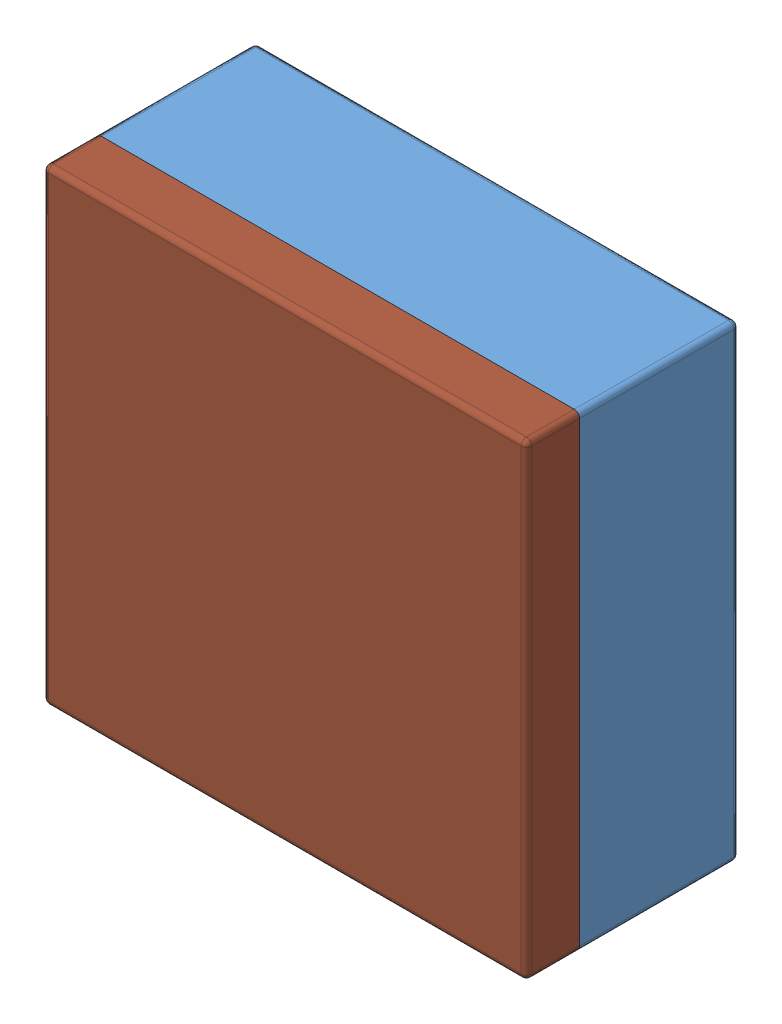
SolidWorks assembly Assem1, configuration Default. Lengths in mm.
Overall size (91 88 40).
617 component instances, 138 part files, 2 mates.
Components (placement in the parent):
- Assem147-1: Assem147 [Default] at (118.0608 24.9039 43.2392) size (91 88 30)
  - 2nd below-1: 2nd below [Default] at (-134.3508 -23.6695 15.6533) size (91 88 30)
  - Main Controller.step-1: Main Controller.step [Default] at (-5.5498 -47.3965 22.6108) x (0 1 0) z (0 0 1) size (83.62 86.87 19.5)
    - Board.step-1: Board.step [Default] at origin size (78.99 86.87 0.41)
      - Open CASCADE STEP translator 6.8 1.1.1.step-1: Open CASCADE STEP translator 6.8 1.1.1.step [Default] at (0 0 -0.4115) size (78.99 86.87 0.41)
    - IC2.step-1: IC2.step [Default] at origin size (3 4.93 1.1)
      - 6352354192.step-1: 6352354192.step [Default] at (37.973 87.63 0.69) x (1 0 0) z (0 -1 0) size (3 1.1 4.93)
        - BODY-SO.step-1: BODY-SO.step [Default] at origin size (3 1 3)
        - LEAD-SO.step-1: LEAD-SO.step [Default] at (1 -0.44 1.9) size (0.22 0.69 0.96)
        - LEAD-SO.step-2: LEAD-SO.step [Default] at (0.5 -0.44 1.9) size (0.22 0.69 0.96)
        - LEAD-SO.step-3: LEAD-SO.step [Default] at (0 -0.44 1.9) size (0.22 0.69 0.96)
        - LEAD-SO.step-4: LEAD-SO.step [Default] at (-0.5 -0.44 1.9) size (0.22 0.69 0.96)
        - LEAD-SO.step-5: LEAD-SO.step [Default] at (-1 -0.44 1.9) size (0.22 0.69 0.96)
        - LEAD-SO.step-6: LEAD-SO.step [Default] at (1 -0.44 -1.9) x (-1 0 0) z (0 0 -1) size (0.22 0.69 0.96)
        - LEAD-SO.step-7: LEAD-SO.step [Default] at (0.5 -0.44 -1.9) x (-1 0 0) z (0 0 -1) size (0.22 0.69 0.96)
        - LEAD-SO.step-8: LEAD-SO.step [Default] at (0 -0.44 -1.9) x (-1 0 0) z (0 0 -1) size (0.22 0.69 0.96)
        - LEAD-SO.step-9: LEAD-SO.step [Default] at (-0.5 -0.44 -1.9) x (-1 0 0) z (0 0 -1) size (0.22 0.69 0.96)
        - LEAD-SO.step-10: LEAD-SO.step [Default] at (-1 -0.44 -1.9) x (-1 0 0) z (0 0 -1) size (0.22 0.69 0.96)
    - S2.step-1: S2.step [Default] at origin size (4.38 3.7 1.8)
      - 6352354672.step-1: 6352354672.step [Default] at (30.053 53.017 0) size (4.38 3.7 1.8)
        - Body.step-1: Body.step [Default] at (0 0 0.1) size (3.82 3.4 1.7)
        - Pins.step-1: Pins.step [Default] at origin size (4.38 3.7 0.1)
    - S1.step-1: S1.step [Default] at origin size (4.38 3.7 1.8)
      - 6352354672.step-1: 6352354672.step [Default] at (30.053 62.1012 0) size (4.38 3.7 1.8)
        - Body.step-1: Body.step [Default] at (0 0 0.1) size (3.82 3.4 1.7)
        - Pins.step-1: Pins.step [Default] at origin size (4.38 3.7 0.1)
    - DS2.step-1: DS2.step [Default] at origin size (1.6 0.8 0.9)
      - 6357174448.step-1: 6357174448.step [Default] at (51.31 84.836 0.4) size (1.1 0.8 0.5)
        - Extruded.step-1: Extruded.step [Default] at origin size (1.1 0.8 0.5)
      - 6357174288.step-1: 6357174288.step [Default] at (51.31 84.836 0) size (1.6 0.8 0.4)
        - Extruded-0.step-1: Extruded-0.step [Default] at origin size (1.6 0.8 0.4)
    - DS1.step-1: DS1.step [Default] at origin size (0.8 1.6 0.9)
      - 6357175488.step-1: 6357175488.step [Default] at (71.8819 81.917 0.4) size (0.8 1.1 0.5)
        - Extruded-1.step-1: Extruded-1.step [Default] at origin size (0.8 1.1 0.5)
      - 6357175328.step-1: 6357175328.step [Default] at (71.8819 81.917 0) size (0.8 1.6 0.4)
        - Extruded-2.step-1: Extruded-2.step [Default] at origin size (0.8 1.6 0.4)
    - P1.step-1: P1.step [Default] at origin size (7.9 4.5 9.4)
      - 6357176688.step-1: 6357176688.step [Default] at (78.67 45.298 0) size (3.15 1.45 6)
        - Extruded-3.step-1: Extruded-3.step [Default] at origin size (3.15 1.45 6)
      - 6357176528.step-1: 6357176528.step [Default] at (79.92 44.173 0) size (0.65 0.8 4.1)
        - Extruded-4.step-1: Extruded-4.step [Default] at origin size (0.65 0.8 4.1)
      - 6357176528.step-2: 6357176528.step [Default] at (72.67 44.173 0) size (0.65 0.8 4.1)
        - Extruded-4.step-1: Extruded-4.step [Default] at origin size (0.65 0.8 4.1)
      - 6357176288.step-1: 6357176288.step [Default] at (73.92 45.298 0) size (3.15 1.45 6)
        - Extruded-5.step-1: Extruded-5.step [Default] at origin size (3.15 1.45 6)
      - 6357176128.step-1: 6357176128.step [Default] at (76.295 42.648 0) size (7.9 2.25 6)
        - Extruded-6.step-1: Extruded-6.step [Default] at origin size (7.9 2.25 6)
      - 6357175968.step-1: 6357175968.step [Default] at (76.295 43.973 0) size (6.6 4.1 1.75)
        - Extruded-7.step-1: Extruded-7.step [Default] at origin size (6.6 4.1 1.75)
      - 6357175808.step-1: 6357175808.step [Default] at (76.295 44.323 -3.4) size (0.5 0.5 8.45)
        - Extruded-8.step-1: Extruded-8.step [Default] at origin size (0.5 0.5 8.45)
      - 6357175808.step-2: 6357175808.step [Default] at (74.295 44.323 -3.4) size (0.5 0.5 8.45)
        - Extruded-8.step-1: Extruded-8.step [Default] at origin size (0.5 0.5 8.45)
      - 6357175808.step-3: 6357175808.step [Default] at (78.295 44.323 -3.4) size (0.5 0.5 8.45)
        - Extruded-8.step-1: Extruded-8.step [Default] at origin size (0.5 0.5 8.45)
    - P2.step-1: P2.step [Default] at origin size (7.9 4.5 9.4)
      - 6357176688.step-1: 6357176688.step [Default] at (64.478 45.213 0) size (3.15 1.45 6)
        - Extruded-3.step-1: Extruded-3.step [Default] at origin size (3.15 1.45 6)
      - 6357176528.step-1: 6357176528.step [Default] at (65.728 44.088 0) size (0.65 0.8 4.1)
        - Extruded-4.step-1: Extruded-4.step [Default] at origin size (0.65 0.8 4.1)
      - 6357176528.step-2: 6357176528.step [Default] at (58.478 44.088 0) size (0.65 0.8 4.1)
        - Extruded-4.step-1: Extruded-4.step [Default] at origin size (0.65 0.8 4.1)
      - 6357176288.step-1: 6357176288.step [Default] at (59.728 45.213 0) size (3.15 1.45 6)
        - Extruded-5.step-1: Extruded-5.step [Default] at origin size (3.15 1.45 6)
      - 6357176128.step-1: 6357176128.step [Default] at (62.103 42.563 0) size (7.9 2.25 6)
        - Extruded-6.step-1: Extruded-6.step [Default] at origin size (7.9 2.25 6)
      - 6357175968.step-1: 6357175968.step [Default] at (62.103 43.888 0) size (6.6 4.1 1.75)
        - Extruded-7.step-1: Extruded-7.step [Default] at origin size (6.6 4.1 1.75)
      - 6357175808.step-1: 6357175808.step [Default] at (62.103 44.238 -3.4) size (0.5 0.5 8.45)
        - Extruded-8.step-1: Extruded-8.step [Default] at origin size (0.5 0.5 8.45)
      - 6357175808.step-2: 6357175808.step [Default] at (60.103 44.238 -3.4) size (0.5 0.5 8.45)
        - Extruded-8.step-1: Extruded-8.step [Default] at origin size (0.5 0.5 8.45)
      - 6357175808.step-3: 6357175808.step [Default] at (64.103 44.238 -3.4) size (0.5 0.5 8.45)
        - Extruded-8.step-1: Extruded-8.step [Default] at origin size (0.5 0.5 8.45)
    - K1.step-1: K1.step [Default] at origin size (15 19 19.5)
      - 6352352272.step-1: 6352352272.step [Default] at (79.2542 59.744 15.04) x (0 1 0) z (0 0 -1) size (19 15 19.5)
    - K2.step-1: K2.step [Default] at origin size (15 19 19.5)
      - 6352352272.step-1: 6352352272.step [Default] at (63.246 59.744 15.04) x (0 1 0) z (0 0 -1) size (19 15 19.5)
    - U5.step-1: U5.step [Default] at origin size (6.42 7.8 1)
      - PW0024AakaMTC24.step-1: PW0024AakaMTC24.step [Default] at (53.9751 104.7751 0.624) x (0 1 0) z (1 0 0) size (7.8 1 6.42)
        - BODY_MTC24.step-1: BODY_MTC24.step [Default] at origin size (7.8 0.9 4.4)
        - LEAD_MTC24.step-1: LEAD_MTC24.step [Default] at (3.575 -0.3725 -2.6) x (-1 0 0) z (0 0 -1) size (0.24 0.62 1.01)
        - LEAD_MTC24.step-2: LEAD_MTC24.step [Default] at (2.925 -0.3725 -2.6) x (-1 0 0) z (0 0 -1) size (0.24 0.62 1.01)
        - LEAD_MTC24.step-3: LEAD_MTC24.step [Default] at (2.275 -0.3725 -2.6) x (-1 0 0) z (0 0 -1) size (0.24 0.62 1.01)
        - LEAD_MTC24.step-4: LEAD_MTC24.step [Default] at (1.625 -0.3725 -2.6) x (-1 0 0) z (0 0 -1) size (0.24 0.62 1.01)
        - LEAD_MTC24.step-5: LEAD_MTC24.step [Default] at (0.975 -0.3725 -2.6) x (-1 0 0) z (0 0 -1) size (0.24 0.62 1.01)
        - LEAD_MTC24.step-6: LEAD_MTC24.step [Default] at (0.325 -0.3725 -2.6) x (-1 0 0) z (0 0 -1) size (0.24 0.62 1.01)
        - LEAD_MTC24.step-7: LEAD_MTC24.step [Default] at (-0.325 -0.3725 -2.6) x (-1 0 0) z (0 0 -1) size (0.24 0.62 1.01)
        - LEAD_MTC24.step-8: LEAD_MTC24.step [Default] at (-0.975 -0.3725 -2.6) x (-1 0 0) z (0 0 -1) size (0.24 0.62 1.01)
        - LEAD_MTC24.step-9: LEAD_MTC24.step [Default] at (-1.625 -0.3725 -2.6) x (-1 0 0) z (0 0 -1) size (0.24 0.62 1.01)
        - LEAD_MTC24.step-10: LEAD_MTC24.step [Default] at (-2.275 -0.3725 -2.6) x (-1 0 0) z (0 0 -1) size (0.24 0.62 1.01)
        - LEAD_MTC24.step-11: LEAD_MTC24.step [Default] at (-2.925 -0.3725 -2.6) x (-1 0 0) z (0 0 -1) size (0.24 0.62 1.01)
        - LEAD_MTC24.step-12: LEAD_MTC24.step [Default] at (-3.575 -0.3725 -2.6) x (-1 0 0) z (0 0 -1) size (0.24 0.62 1.01)
        - LEAD_MTC24.step-13: LEAD_MTC24.step [Default] at (3.575 -0.3725 2.6) size (0.24 0.62 1.01)
        - LEAD_MTC24.step-14: LEAD_MTC24.step [Default] at (2.925 -0.3725 2.6) size (0.24 0.62 1.01)
        - LEAD_MTC24.step-15: LEAD_MTC24.step [Default] at (2.275 -0.3725 2.6) size (0.24 0.62 1.01)
        - LEAD_MTC24.step-16: LEAD_MTC24.step [Default] at (1.625 -0.3725 2.6) size (0.24 0.62 1.01)
        - LEAD_MTC24.step-17: LEAD_MTC24.step [Default] at (0.975 -0.3725 2.6) size (0.24 0.62 1.01)
        - LEAD_MTC24.step-18: LEAD_MTC24.step [Default] at (0.325 -0.3725 2.6) size (0.24 0.62 1.01)
        - LEAD_MTC24.step-19: LEAD_MTC24.step [Default] at (-0.325 -0.3725 2.6) size (0.24 0.62 1.01)
        - LEAD_MTC24.step-20: LEAD_MTC24.step [Default] at (-0.975 -0.3725 2.6) size (0.24 0.62 1.01)
        - LEAD_MTC24.step-21: LEAD_MTC24.step [Default] at (-1.625 -0.3725 2.6) size (0.24 0.62 1.01)
        - LEAD_MTC24.step-22: LEAD_MTC24.step [Default] at (-2.275 -0.3725 2.6) size (0.24 0.62 1.01)
        - LEAD_MTC24.step-23: LEAD_MTC24.step [Default] at (-2.925 -0.3725 2.6) size (0.24 0.62 1.01)
        - LEAD_MTC24.step-24: LEAD_MTC24.step [Default] at (-3.575 -0.3725 2.6) size (0.24 0.62 1.01)
    - U4.step-1: U4.step [Default] at origin size (4.9 6 1.76)
      - IC_Texas_Instruments_ISO7220ADR_eec.step-1: IC_Texas_Instruments_ISO7220ADR_eec.step [Default] at (51.943 77.597 0) x (0 1 0) z (0 0 1) size (6 4.9 1.76)
        - IC_BODY.step-1: IC_BODY.step [Default] at (0 0 0.25) x (0 -1 0) z (0 0 1) size (4.9 3.9 1.5)
        - circle.step-1: circle.step [Default] at (-1.0726 1.9393 1.751) x (1 0 0) z (0 0 -1) size (0.4 0.4 0)
        - IC_LEG.step-1: IC_LEG.step [Default] at (-3 2.1095 0) x (1 0 0) z (0 -1 0) size (1.15 1.11 0.41)
        - IC_LEG.step-2: IC_LEG.step [Default] at (-3 0.8395 0) x (1 0 0) z (0 -1 0) size (1.15 1.11 0.41)
        - IC_LEG.step-3: IC_LEG.step [Default] at (-3 -0.4305 0) x (1 0 0) z (0 -1 0) size (1.15 1.11 0.41)
        - IC_LEG.step-4: IC_LEG.step [Default] at (-3 -1.7005 0) x (1 0 0) z (0 -1 0) size (1.15 1.11 0.41)
        - Texas_Instruments.step-1: Texas_Instruments.step [Default] at (0.0232 -1.7093 1.75) size (3.04 0.71 0.02)
        - IC_LEG_MIR8.step-1: IC_LEG_MIR8.step [Default] at (3 2.1095 0) x (-1 0 0) z (0 1 0) size (1.15 1.11 0.41)
        - IC_LEG_MIR8.step-2: IC_LEG_MIR8.step [Default] at (3 0.8395 0) x (-1 0 0) z (0 1 0) size (1.15 1.11 0.41)
        - IC_LEG_MIR8.step-3: IC_LEG_MIR8.step [Default] at (3 -0.4305 0) x (-1 0 0) z (0 1 0) size (1.15 1.11 0.41)
        - IC_LEG_MIR8.step-4: IC_LEG_MIR8.step [Default] at (3 -1.7005 0) x (-1 0 0) z (0 1 0) size (1.15 1.11 0.41)
    - U3.step-1: U3.step [Default] at origin size (7.05 6.5 1.8)
      - IC_Advanced_Monolithic_Systems_AMS1117-3_3_eec.step-1: IC_Advanced_Monolithic_Systems_AMS1117-3_3_eec.step [Default] at (38.227 106.68 0) size (7.05 6.51 1.8)
        - 2.step-1: 2.step [Default] x (1 0 0) z (0 -1 0) size (7.05 1.2 5.34)
          - Open CASCADE STEP translator 6.8 1.13.1.2.1.step-1: Open CASCADE STEP translator 6.8 1.13.1.2.1.step [Default] at origin size (7.05 1.2 5.34)
          - Open CASCADE STEP translator 6.8 1.13.1.2.2.step-1: Open CASCADE STEP translator 6.8 1.13.1.2.2.step [Default] at origin
        - 1.step-1: 1.step [Default] at (0 0 0.74) x (0 1 0) z (0 0 1) size (6.51 3.5 1.06)
        - Notch_2.step-1: Notch_2.step [Default] at (-0.7251 1.7063 1.701) size (2.3 5.16 0.1)
    - U2.step-1: U2.step [Default] at origin size (4.9 6 1.63)
      - SOIC-8akaD0008AakaM08A.step-1: SOIC-8akaD0008AakaM08A.step [Default] at (69.5961 112.9199 1) x (1 0 0) z (0 -1 0) size (4.9 1.63 6)
        - M08A_ASM_82_ASM.step-1: M08A_ASM_82_ASM.step [Default] at origin size (4.9 1.63 6)
          - TIEBAR_M08A_2_ASM.step-1: TIEBAR_M08A_2_ASM.step [Default] at origin size (4.9 0.2 0.66)
            - MANIFOLD_SOLID_BREP_2784.step-1: MANIFOLD_SOLID_BREP_2784.step [Default] at origin size (0.2 0.2 0.15)
            - MANIFOLD_SOLID_BREP_2935.step-1: MANIFOLD_SOLID_BREP_2935.step [Default] at origin size (0.2 0.2 0.15)
            - MANIFOLD_SOLID_BREP_3086.step-1: MANIFOLD_SOLID_BREP_3086.step [Default] at origin size (0.2 0.2 0.15)
            - MANIFOLD_SOLID_BREP_3237.step-1: MANIFOLD_SOLID_BREP_3237.step [Default] at origin size (0.2 0.2 0.15)
          - BODY_M08A_35.step-1: BODY_M08A_35.step [Default] at origin size (4.9 1.45 3.9)
          - LEAD_M08A_57.step-1: LEAD_M08A_57.step [Default] at (1.905 -0.75 2.1732) size (0.38 1 1.05)
          - LEAD_M08A_57.step-2: LEAD_M08A_57.step [Default] at (0.635 -0.75 2.1732) size (0.38 1 1.05)
          - LEAD_M08A_57.step-3: LEAD_M08A_57.step [Default] at (-0.635 -0.75 2.1732) size (0.38 1 1.05)
          - LEAD_M08A_57.step-4: LEAD_M08A_57.step [Default] at (-1.905 -0.75 2.1732) size (0.38 1 1.05)
          - LEAD_M08A_57.step-5: LEAD_M08A_57.step [Default] at (1.905 -0.75 -2.1732) x (-1 0 0) z (0 0 -1) size (0.38 1 1.05)
          - LEAD_M08A_57.step-6: LEAD_M08A_57.step [Default] at (0.635 -0.75 -2.1732) x (-1 0 0) z (0 0 -1) size (0.38 1 1.05)
          - LEAD_M08A_57.step-7: LEAD_M08A_57.step [Default] at (-0.635 -0.75 -2.1732) x (-1 0 0) z (0 0 -1) size (0.38 1 1.05)
          - LEAD_M08A_57.step-8: LEAD_M08A_57.step [Default] at (-1.905 -0.75 -2.1732) x (-1 0 0) z (0 0 -1) size (0.38 1 1.05)
    - U1.step-1: U1.step [Default] at origin size (2.01 3.1 0.92)
      - IC_Texas_Instruments_TXS0102DCUR_eec.step-1: IC_Texas_Instruments_TXS0102DCUR_eec.step [Default] at (54.737 114.495 0) x (0 1 0) z (0 0 1) size (0.25 1.32 0.01)
      - IC_Texas_Instruments_TXS0102DCUR_eec-9.step-1: IC_Texas_Instruments_TXS0102DCUR_eec-9.step [Default] at (54.737 114.495 0) x (0 1 0) z (0 0 1) size (0.19 0.66 0.01)
      - IC_Texas_Instruments_TXS0102DCUR_eec-10.step-1: IC_Texas_Instruments_TXS0102DCUR_eec-10.step [Default] at (54.737 114.495 0) x (0 1 0) z (0 0 1) size (0.19 1.33 0.01)
      - IC_Texas_Instruments_TXS0102DCUR_eec-11.step-1: IC_Texas_Instruments_TXS0102DCUR_eec-11.step [Default] at (54.737 114.495 0) x (0 1 0) z (0 0 1) size (0.3 0.3 0.01)
      - IC_Texas_Instruments_TXS0102DCUR_eec-12.step-1: IC_Texas_Instruments_TXS0102DCUR_eec-12.step [Default] at (54.737 114.495 0) x (0 1 0) z (0 0 1) size (3.1 1.71 0.56)
      - IC_Texas_Instruments_TXS0102DCUR_eec-13.step-1: IC_Texas_Instruments_TXS0102DCUR_eec-13.step [Default] at (54.737 114.495 0) x (0 1 0) z (0 0 1) size (2.31 2.01 0.8)
    - R23.step-1: R23.step [Default] at origin size (0.8 1.6 0.56)
      - Res_Panasonic_Electronic_Components_ERA-3ARB202V_eec.step-1: Res_Panasonic_Electronic_Components_ERA-3ARB202V_eec.step [Default] at (70.739 75.309 0) x (0 -1 0) z (0 0 1) size (1.6 0.8 0.56)
        - 1-14.step-1: 1-14.step [Default] at origin size (1.52 0.8 0.47)
        - 2-15.step-1: 2-15.step [Default] at origin size (1.08 0.8 0.04)
        - 3.step-1: 3.step [Default] at origin size (1.6 0.8 0.55)
        - Panasonic_Logo.step-1: Panasonic_Logo.step [Default] at (-0.1032 0.2046 0.451) size (0.41 0.06 0.11)
    - R22.step-1: R22.step [Default] at origin size (0.8 1.6 0.56)
      - Res_Panasonic_Electronic_Components_ERA-3ARB202V_eec.step-1: Res_Panasonic_Electronic_Components_ERA-3ARB202V_eec.step [Default] at (68.453 75.309 0) x (0 -1 0) z (0 0 1) size (1.6 0.8 0.56)
        - 1-14.step-1: 1-14.step [Default] at origin size (1.52 0.8 0.47)
        - 2-15.step-1: 2-15.step [Default] at origin size (1.08 0.8 0.04)
        - 3.step-1: 3.step [Default] at origin size (1.6 0.8 0.55)
        - Panasonic_Logo.step-1: Panasonic_Logo.step [Default] at (-0.1032 0.2046 0.451) size (0.41 0.06 0.11)
    - R21.step-1: R21.step [Default] at origin size (0.95 1.75 0.55)
      - 6357174128.step-1: 6357174128.step [Default] at (66.167 75.184 0) size (0.95 1.15 0.55)
        - Extruded-16.step-1: Extruded-16.step [Default] at origin size (0.95 1.15 0.55)
      - 6357173968.step-1: 6357173968.step [Default] at (66.167 74.459 0) size (0.95 0.3 0.55)
        - Extruded-17.step-1: Extruded-17.step [Default] at origin size (0.95 0.3 0.55)
      - 6357173968.step-2: 6357173968.step [Default] at (66.167 75.909 0) size (0.95 0.3 0.55)
        - Extruded-17.step-1: Extruded-17.step [Default] at origin size (0.95 0.3 0.55)
    - R20.step-1: R20.step [Default] at origin size (0.95 1.75 0.55)
      - 6357174128.step-1: 6357174128.step [Default] at (62.992 77.637 0) size (0.95 1.15 0.55)
        - Extruded-16.step-1: Extruded-16.step [Default] at origin size (0.95 1.15 0.55)
      - 6357173968.step-1: 6357173968.step [Default] at (62.992 78.362 0) size (0.95 0.3 0.55)
        - Extruded-17.step-1: Extruded-17.step [Default] at origin size (0.95 0.3 0.55)
      - 6357173968.step-2: 6357173968.step [Default] at (62.992 76.912 0) size (0.95 0.3 0.55)
        - Extruded-17.step-1: Extruded-17.step [Default] at origin size (0.95 0.3 0.55)
    - R19.step-1: R19.step [Default] at origin size (0.55 1.05 0.4)
      - 6352344032.step-1: 6352344032.step [Default] at (58.42 97.3481 0) x (0 -1 0) z (0 0 1) size (1.05 0.55 0.4)
        - Terminal.step-1: Terminal.step [Default] at (-0.525 -0.275 0) size (0.2 0.55 0.4)
          - Open_CASCADE_STEP_translator_6.8_9.2.1.step-1: Open_CASCADE_STEP_translator_6.8_9.2.1.step [Default] at origin size (0.2 0.55 0.4)
        - Terminal.step-2: Terminal.step [Default] at (0.525 0.275 0) x (-1 0 0) z (0 0 1) size (0.2 0.55 0.4)
          - Open_CASCADE_STEP_translator_6.8_9.2.1.step-1: Open_CASCADE_STEP_translator_6.8_9.2.1.step [Default] at origin size (0.2 0.55 0.4)
        - Mid_Body.step-1: Mid_Body.step [Default] at (-0.525 -0.275 0) size (0.97 0.55 0.32)
        - Mark.step-1: Mark.step [Default] at (-0.325 -0.275 0.36) size (0.65 0.55 0.04)
    - R18.step-1: R18.step [Default] at origin size (0.55 1.05 0.4)
      - 6352344032.step-1: 6352344032.step [Default] at (56.9828 97.3481 0) x (0 -1 0) z (0 0 1) size (1.05 0.55 0.4)
        - Terminal.step-1: Terminal.step [Default] at (-0.525 -0.275 0) size (0.2 0.55 0.4)
          - Open_CASCADE_STEP_translator_6.8_9.2.1.step-1: Open_CASCADE_STEP_translator_6.8_9.2.1.step [Default] at origin size (0.2 0.55 0.4)
        - Terminal.step-2: Terminal.step [Default] at (0.525 0.275 0) x (-1 0 0) z (0 0 1) size (0.2 0.55 0.4)
          - Open_CASCADE_STEP_translator_6.8_9.2.1.step-1: Open_CASCADE_STEP_translator_6.8_9.2.1.step [Default] at origin size (0.2 0.55 0.4)
        - Mid_Body.step-1: Mid_Body.step [Default] at (-0.525 -0.275 0) size (0.97 0.55 0.32)
        - Mark.step-1: Mark.step [Default] at (-0.325 -0.275 0.36) size (0.65 0.55 0.04)
    - R17.step-1: R17.step [Default] at origin size (0.8 1.6 0.56)
      - Res_Panasonic_Electronic_Components_ERA-3ARB202V_eec.step-1: Res_Panasonic_Electronic_Components_ERA-3ARB202V_eec.step [Default] at (55.118 96.8731 0) x (0 -1 0) z (0 0 1) size (1.6 0.8 0.56)
        - 1-14.step-1: 1-14.step [Default] at origin size (1.52 0.8 0.47)
        - 2-15.step-1: 2-15.step [Default] at origin size (1.08 0.8 0.04)
        - 3.step-1: 3.step [Default] at origin size (1.6 0.8 0.55)
        - Panasonic_Logo.step-1: Panasonic_Logo.step [Default] at (-0.1032 0.2046 0.451) size (0.41 0.06 0.11)
    - R16.step-1: R16.step [Default] at origin size (3.4 2.7 0.7)
      - 6357171968.step-1: 6357171968.step [Default] at (37.973 78.486 0) size (2.4 2.7 0.7)
        - Extruded-18.step-1: Extruded-18.step [Default] at origin size (2.4 2.7 0.7)
      - 6357171808.step-1: 6357171808.step [Default] at (36.523 78.486 0) size (0.5 2.7 0.7)
        - Extruded-19.step-1: Extruded-19.step [Default] at origin size (0.5 2.7 0.7)
      - 6357171808.step-2: 6357171808.step [Default] at (39.423 78.486 0) size (0.5 2.7 0.7)
        - Extruded-19.step-1: Extruded-19.step [Default] at origin size (0.5 2.7 0.7)
    - R15.step-1: R15.step [Default] at origin size (0.55 1.05 0.4)
      - 6352344032.step-1: 6352344032.step [Default] at (66.548 97.376 0) x (0 -1 0) z (0 0 1) size (1.05 0.55 0.4)
        - Terminal.step-1: Terminal.step [Default] at (-0.525 -0.275 0) size (0.2 0.55 0.4)
          - Open_CASCADE_STEP_translator_6.8_9.2.1.step-1: Open_CASCADE_STEP_translator_6.8_9.2.1.step [Default] at origin size (0.2 0.55 0.4)
        - Terminal.step-2: Terminal.step [Default] at (0.525 0.275 0) x (-1 0 0) z (0 0 1) size (0.2 0.55 0.4)
          - Open_CASCADE_STEP_translator_6.8_9.2.1.step-1: Open_CASCADE_STEP_translator_6.8_9.2.1.step [Default] at origin size (0.2 0.55 0.4)
        - Mid_Body.step-1: Mid_Body.step [Default] at (-0.525 -0.275 0) size (0.97 0.55 0.32)
        - Mark.step-1: Mark.step [Default] at (-0.325 -0.275 0.36) size (0.65 0.55 0.04)
    - R14.step-1: R14.step [Default] at origin size (0.55 1.05 0.4)
      - 6352344032.step-1: 6352344032.step [Default] at (65.1496 97.376 0) x (0 -1 0) z (0 0 1) size (1.05 0.55 0.4)
        - Terminal.step-1: Terminal.step [Default] at (-0.525 -0.275 0) size (0.2 0.55 0.4)
          - Open_CASCADE_STEP_translator_6.8_9.2.1.step-1: Open_CASCADE_STEP_translator_6.8_9.2.1.step [Default] at origin size (0.2 0.55 0.4)
        - Terminal.step-2: Terminal.step [Default] at (0.525 0.275 0) x (-1 0 0) z (0 0 1) size (0.2 0.55 0.4)
          - Open_CASCADE_STEP_translator_6.8_9.2.1.step-1: Open_CASCADE_STEP_translator_6.8_9.2.1.step [Default] at origin size (0.2 0.55 0.4)
        - Mid_Body.step-1: Mid_Body.step [Default] at (-0.525 -0.275 0) size (0.97 0.55 0.32)
        - Mark.step-1: Mark.step [Default] at (-0.325 -0.275 0.36) size (0.65 0.55 0.04)
    - R13.step-1: R13.step [Default] at origin size (3.4 2.7 0.7)
      - 6357171968.step-1: 6357171968.step [Default] at (37.973 81.915 0) size (2.4 2.7 0.7)
        - Extruded-18.step-1: Extruded-18.step [Default] at origin size (2.4 2.7 0.7)
      - 6357171808.step-1: 6357171808.step [Default] at (39.423 81.915 0) size (0.5 2.7 0.7)
        - Extruded-19.step-1: Extruded-19.step [Default] at origin size (0.5 2.7 0.7)
      - 6357171808.step-2: 6357171808.step [Default] at (36.523 81.915 0) size (0.5 2.7 0.7)
        - Extruded-19.step-1: Extruded-19.step [Default] at origin size (0.5 2.7 0.7)
    - R12.step-1: R12.step [Default] at origin size (2.2 1.45 0.7)
      - 6357172608.step-1: 6357172608.step [Default] at (62.611 104.0312 0) size (1.4 1.45 0.7)
        - Extruded-20.step-1: Extruded-20.step [Default] at origin size (1.4 1.45 0.7)
      - 6357172448.step-1: 6357172448.step [Default] at (61.711 104.0312 0) size (0.4 1.45 0.7)
        - Extruded-21.step-1: Extruded-21.step [Default] at origin size (0.4 1.45 0.7)
      - 6357172448.step-2: 6357172448.step [Default] at (63.511 104.0312 0) size (0.4 1.45 0.7)
        - Extruded-21.step-1: Extruded-21.step [Default] at origin size (0.4 1.45 0.7)
    - R11.step-1: R11.step [Default] at origin size (2.2 1.45 0.7)
      - 6357172608.step-1: 6357172608.step [Default] at (62.611 101.727 0) size (1.4 1.45 0.7)
        - Extruded-20.step-1: Extruded-20.step [Default] at origin size (1.4 1.45 0.7)
      - 6357172448.step-1: 6357172448.step [Default] at (61.711 101.727 0) size (0.4 1.45 0.7)
        - Extruded-21.step-1: Extruded-21.step [Default] at origin size (0.4 1.45 0.7)
      - 6357172448.step-2: 6357172448.step [Default] at (63.511 101.727 0) size (0.4 1.45 0.7)
        - Extruded-21.step-1: Extruded-21.step [Default] at origin size (0.4 1.45 0.7)
    - R10.step-1: R10.step [Default] at origin size (1.75 0.95 0.55)
      - 6352350352.step-1: 6352350352.step [Default] at (51.435 87.2253 0) size (1.75 0.95 0.55)
        - Terminal-1.step-1: Terminal-1.step [Default] at (-0.875 -0.475 0) size (0.15 0.95 0.55)
          - Open_CASCADE_STEP_translator_6.8_2.2.1.step-1: Open_CASCADE_STEP_translator_6.8_2.2.1.step [Default] at origin size (0.15 0.95 0.55)
        - Terminal-1.step-2: Terminal-1.step [Default] at (0.875 0.475 0) x (-1 0 0) z (0 0 1) size (0.15 0.95 0.55)
          - Open_CASCADE_STEP_translator_6.8_2.2.1.step-1: Open_CASCADE_STEP_translator_6.8_2.2.1.step [Default] at origin size (0.15 0.95 0.55)
        - Mid_Body-22.step-1: Mid_Body-22.step [Default] at (-0.875 -0.475 0) size (1.64 0.95 0.44)
        - Mark-23.step-1: Mark-23.step [Default] at (-0.725 -0.475 0.495) size (1.45 0.95 0.06)
    - R9.step-1: R9.step [Default] at origin size (0.8 1.6 0.56)
      - Res_Panasonic_Electronic_Components_ERA-3AEB3652V_eec.step-1: Res_Panasonic_Electronic_Components_ERA-3AEB3652V_eec.step [Default] at (62.5855 96.52 0) x (0 1 0) z (0 0 1) size (1.6 0.8 0.56)
        - 1-24.step-1: 1-24.step [Default] at origin size (1.52 0.8 0.47)
        - 2-25.step-1: 2-25.step [Default] at origin size (1.08 0.8 0.04)
        - 3-26.step-1: 3-26.step [Default] at origin size (1.6 0.8 0.55)
        - Panasonic_Logo-27.step-1: Panasonic_Logo-27.step [Default] at (-0.1032 0.2046 0.451) size (0.41 0.06 0.11)
    - R8.step-1: R8.step [Default] at origin size (0.8 1.6 0.56)
      - Res_Panasonic_Electronic_Components_ERA-3AEB3652V_eec.step-1: Res_Panasonic_Electronic_Components_ERA-3AEB3652V_eec.step [Default] at (60.325 96.52 0) x (0 1 0) z (0 0 1) size (1.6 0.8 0.56)
        - 1-24.step-1: 1-24.step [Default] at origin size (1.52 0.8 0.47)
        - 2-25.step-1: 2-25.step [Default] at origin size (1.08 0.8 0.04)
        - 3-26.step-1: 3-26.step [Default] at origin size (1.6 0.8 0.55)
        - Panasonic_Logo-27.step-1: Panasonic_Logo-27.step [Default] at (-0.1032 0.2046 0.451) size (0.41 0.06 0.11)
    - R7.step-1: R7.step [Default] at origin size (1.75 0.95 0.55)
      - 6352350352.step-1: 6352350352.step [Default] at (51.435 89.6295 0) size (1.75 0.95 0.55)
        - Terminal-1.step-1: Terminal-1.step [Default] at (-0.875 -0.475 0) size (0.15 0.95 0.55)
          - Open_CASCADE_STEP_translator_6.8_2.2.1.step-1: Open_CASCADE_STEP_translator_6.8_2.2.1.step [Default] at origin size (0.15 0.95 0.55)
        - Terminal-1.step-2: Terminal-1.step [Default] at (0.875 0.475 0) x (-1 0 0) z (0 0 1) size (0.15 0.95 0.55)
          - Open_CASCADE_STEP_translator_6.8_2.2.1.step-1: Open_CASCADE_STEP_translator_6.8_2.2.1.step [Default] at origin size (0.15 0.95 0.55)
        - Mid_Body-22.step-1: Mid_Body-22.step [Default] at (-0.875 -0.475 0) size (1.64 0.95 0.44)
        - Mark-23.step-1: Mark-23.step [Default] at (-0.725 -0.475 0.495) size (1.45 0.95 0.06)
    - R5.step-1: R5.step [Default] at origin size (1.55 0.85 0.5)
      - Res_Vishay_CRCW06033M90FKEC_eec.step-1: Res_Vishay_CRCW06033M90FKEC_eec.step [Default] at (69.0249 101.727 0) x (-1 0 0) z (0 0 1) size (1.55 0.85 0.5)
        - 1-28.step-1: 1-28.step [Default] at origin size (1.55 0.85 0.5)
        - 2-29.step-1: 2-29.step [Default] at origin size (1.45 0.85 0.4)
        - 3-30.step-1: 3-30.step [Default] at origin size (0.95 0.85 0.05)
        - Vishay_logo_-_Copy.step-1: Vishay_logo_-_Copy.step [Default] at (0.4713 0.3036 0.4001) size (0.15 0.21 0.1)
        - Vishay_logo.step-1: Vishay_logo.step [Default] at (0.4789 0.2998 0.4001) size (0.19 0.04 0.11)
    - R4.step-1: R4.step [Default] at origin size (3.1 1.6 0.65)
      - Res_Yageo_RT1206WRB073K92L_eec.step-1: Res_Yageo_RT1206WRB073K92L_eec.step [Default] at (67.3423 102.9804 -1.1394) x (0 1 0) z (1 0 0) size (1.6 0.65 3.1)
        - RT1206FRE071R3L_Ceramic.step-1: RT1206FRE071R3L_Ceramic.step [Default] at (1.2913 1.4646 2.017) size (1.6 0.45 2.9)
        - RT1206FRE071R3L_Logo.step-1: RT1206FRE071R3L_Logo.step [Default] at (2.8145 1.7896 5.3787) x (0 0 -1) z (1 0 0) size (0.7 0 0.09)
        - RT1206FRE071R3L_Terminal.step-1: RT1206FRE071R3L_Terminal.step [Default] at (1.2913 1.1396 0.917) size (1.6 0.65 0.45)
        - RT1206FRE071R3L_Terminal.step-2: RT1206FRE071R3L_Terminal.step [Default] at (1.2913 1.1396 3.117) x (-1 0 0) z (0 0 -1) size (1.6 0.65 0.45)
        - RT1206FRE071R3L_Coating.step-1: RT1206FRE071R3L_Coating.step [Default] at (1.2913 1.7396 2.017) size (1.6 0.1 2.2)
    - R3.step-1: R3.step [Default] at origin size (0.55 1.05 0.4)
      - 6352352672.step-1: 6352352672.step [Default] at (53.34 97.3481 0) x (0 1 0) z (0 0 1) size (1.05 0.55 0.4)
        - Terminal-2.step-1: Terminal-2.step [Default] at (-0.525 -0.275 0) size (0.2 0.55 0.4)
          - Open_CASCADE_STEP_translator_6.8_9.2.1-31.step-1: Open_CASCADE_STEP_translator_6.8_9.2.1-31.step [Default] at origin size (0.2 0.55 0.4)
        - Terminal-2.step-2: Terminal-2.step [Default] at (0.525 0.275 0) x (-1 0 0) z (0 0 1) size (0.2 0.55 0.4)
          - Open_CASCADE_STEP_translator_6.8_9.2.1-31.step-1: Open_CASCADE_STEP_translator_6.8_9.2.1-31.step [Default] at origin size (0.2 0.55 0.4)
        - Mid_Body-32.step-1: Mid_Body-32.step [Default] at (-0.525 -0.275 0) size (0.97 0.55 0.32)
        - Mark-33.step-1: Mark-33.step [Default] at (-0.325 -0.275 0.36) size (0.65 0.55 0.04)
    - R2.step-1: R2.step [Default] at origin size (0.95 1.75 0.55)
      - 6352348192.step-1: 6352348192.step [Default] at (44.577 114.67 0) x (0 1 0) z (0 0 1) size (1.75 0.95 0.55)
        - Terminal-3.step-1: Terminal-3.step [Default] at (-0.875 -0.475 0) size (0.15 0.95 0.55)
          - Open_CASCADE_STEP_translator_6.8_2.2.1-34.step-1: Open_CASCADE_STEP_translator_6.8_2.2.1-34.step [Default] at origin size (0.15 0.95 0.55)
        - Terminal-3.step-2: Terminal-3.step [Default] at (0.875 0.475 0) x (-1 0 0) z (0 0 1) size (0.15 0.95 0.55)
          - Open_CASCADE_STEP_translator_6.8_2.2.1-34.step-1: Open_CASCADE_STEP_translator_6.8_2.2.1-34.step [Default] at origin size (0.15 0.95 0.55)
        - Mid_Body-35.step-1: Mid_Body-35.step [Default] at (-0.875 -0.475 0) size (1.64 0.95 0.44)
        - Mark-36.step-1: Mark-36.step [Default] at (-0.725 -0.475 0.495) size (1.45 0.95 0.06)
    - Q4.step-1: Q4.step [Default] at origin size (2.82 2.9 1.25)
      - Trans_Alpha_&_Omega_Semiconductor_AO3400A_eec.step-1: Trans_Alpha_&_Omega_Semiconductor_AO3400A_eec.step [Default] at (77.146 114.768 0) x (0 -1 0) z (0 0 1) size (2.9 2.82 1.25)
        - 1-37.step-1: 1-37.step [Default] at (0 0 0.1) size (2.9 1.6 1.15)
        - 2-38.step-1: 2-38.step [Default] x (0 -1 0) z (-1 0 0) size (2.82 0.89 2.3)
        - Alpha_&_Omega_Logo.step-1: Alpha_&_Omega_Logo.step [Default] at (-1.3696 -1.3736 1.151) size (2.29 1.19 0.1)
    - Q3.step-1: Q3.step [Default] at origin size (2.82 2.9 1.25)
      - Trans_Alpha_&_Omega_Semiconductor_AO3400A_eec.step-1: Trans_Alpha_&_Omega_Semiconductor_AO3400A_eec.step [Default] at (90.297 114.768 0) x (0 -1 0) z (0 0 1) size (2.9 2.82 1.25)
        - 1-37.step-1: 1-37.step [Default] at (0 0 0.1) size (2.9 1.6 1.15)
        - 2-38.step-1: 2-38.step [Default] x (0 -1 0) z (-1 0 0) size (2.82 0.89 2.3)
        - Alpha_&_Omega_Logo.step-1: Alpha_&_Omega_Logo.step [Default] at (-1.3696 -1.3736 1.151) size (2.29 1.19 0.1)
    - Q2.step-1: Q2.step [Default] at origin size (2.8 2.95 1.25)
      - 6352342192.step-1: 6352342192.step [Default] at (46.294 108.712 0) size (2.8 2.95 1.25)
        - Body-39.step-1: Body-39.step [Default] at origin size (1.6 2.95 1.19)
        - PinsArrayL.step-1: PinsArrayL.step [Default] at origin size (0.6 2.3 0.67)
        - FilletPinR.step-1: FilletPinR.step [Default] at origin size (0.6 0.4 0.67)
    - Q1.step-1: Q1.step [Default] at origin size (2.8 2.95 1.25)
      - 6352342192.step-1: 6352342192.step [Default] at (80.899 122.301 0) size (2.8 2.95 1.25)
        - Body-39.step-1: Body-39.step [Default] at origin size (1.6 2.95 1.19)
        - PinsArrayL.step-1: PinsArrayL.step [Default] at origin size (0.6 2.3 0.67)
        - FilletPinR.step-1: FilletPinR.step [Default] at origin size (0.6 0.4 0.67)
    - K4.step-1: K4.step [Default] at origin size (4.3 6.8 2.3)
      - 6352340992.step-1: 6352340992.step [Default] at (62.357 112.522 0) x (0 1 0) z (0 0 1) size (6.8 4.3 2.3)
        - Body-40.step-1: Body-40.step [Default] at origin size (4.4 4.3 2.2)
        - PinsArrayLR.step-1: PinsArrayLR.step [Default] at origin size (6.8 2.94 1.25)
    - K3.step-1: K3.step [Default] at origin size (6.8 4.3 2.3)
      - 6352351472.step-1: 6352351472.step [Default] at (71.374 88.011 0) x (1 0 0) z (0 0 1) size (6.8 4.3 2.3)
        - Body-41.step-1: Body-41.step [Default] at origin size (4.4 4.3 2.2)
        - PinsArrayLR-42.step-1: PinsArrayLR-42.step [Default] at origin size (6.8 2.94 1.25)
    - JP5.step-1: JP5.step [Default] at origin size (7.4 5.75 10.4)
      - Conn_JST_B2B-XH-A_LF_SN_eec.step-1: Conn_JST_B2B-XH-A_LF_SN_eec.step [Default] at (73.005 121.048 0) x (-1 0 0) z (0 0 1) size (7.4 5.75 10.4)
        - 1-43.step-1: 1-43.step [Default] at (0 0.025 0) x (-1 0 0) z (0 1 0) size (7.4 10.4 5.75)
          - 1-44.step-1: 1-44.step [Default] at origin size (3.14 10.2 0.64)
          - B2B-XH-A.step-1: B2B-XH-A.step [Default] at origin size (7.4 7 5.75)
          - JST_Logo_adjustable.step-1: JST_Logo_adjustable.step [Default] at (-1.7267 5.5034 2.841) size (0.85 2.3 0.01)
    - JP4.step-1: JP4.step [Default] at origin size (12.4 5.75 10.4)
      - Conn_JST_B4B-XH-A_LF_SN_eec.step-1: Conn_JST_B4B-XH-A_LF_SN_eec.step [Default] at (60.833 121.048 0) x (-1 0 0) z (0 0 1) size (12.4 5.75 10.4)
        - 1-45.step-1: 1-45.step [Default] x (1 0 0) z (0 -1 0) size (8.14 10.3 0.9)
        - 2-46.step-1: 2-46.step [Default] x (1 0 0) z (0 -1 0) size (12.4 7 5.75)
        - Pin1_Triangle.step-1: Pin1_Triangle.step [Default] at (-3.7456 -2.776 -1.3492) x (1 0 0) z (0 -1 0) size (0.89 0.61 0.02)
        - JST.step-1: JST.step [Default] at (6.1995 1.4972 0.8858) x (0 1 0) z (1 0 0) size (1.59 0.67 0.01)
    - J9.step-1: J9.step [Default] at origin size (12.4 5.75 10.4)
      - Conn_JST_B4B-XH-A_LF_SN_eec.step-1: Conn_JST_B4B-XH-A_LF_SN_eec.step [Default] at (42.311 53.142 0) x (-1 0 0) z (0 0 1) size (12.4 5.75 10.4)
        - 1-45.step-1: 1-45.step [Default] x (1 0 0) z (0 -1 0) size (8.14 10.3 0.9)
        - 2-46.step-1: 2-46.step [Default] x (1 0 0) z (0 -1 0) size (12.4 7 5.75)
        - Pin1_Triangle.step-1: Pin1_Triangle.step [Default] at (-3.7456 -2.776 -1.3492) x (1 0 0) z (0 -1 0) size (0.89 0.61 0.02)
        - JST.step-1: JST.step [Default] at (6.1995 1.4972 0.8858) x (0 1 0) z (1 0 0) size (1.59 0.67 0.01)
    - J8.step-1: J8.step [Default] at origin size (3.8 20 9.2)
      - Conn_JST_B7B-EH-A_LF_SN_eec.step-1: Conn_JST_B7B-EH-A_LF_SN_eec.step [Default] at (52.405 60.267 0) x (0 -1 0) z (0 0 1) size (20 3.8 9.2)
        - 1-47.step-1: 1-47.step [Default] at (0 0.3 0) x (1 0 0) z (0 -1 0) size (15.64 8 0.64)
        - 2-48.step-1: 2-48.step [Default] at (0 0.3 0) x (1 0 0) z (0 -1 0) size (20 6 3.8)
        - JST-49.step-1: JST-49.step [Default] at (8.5962 -1.9002 0.6223) x (1 0 0) z (0 -1 0) size (1.91 0.8 0.01)
